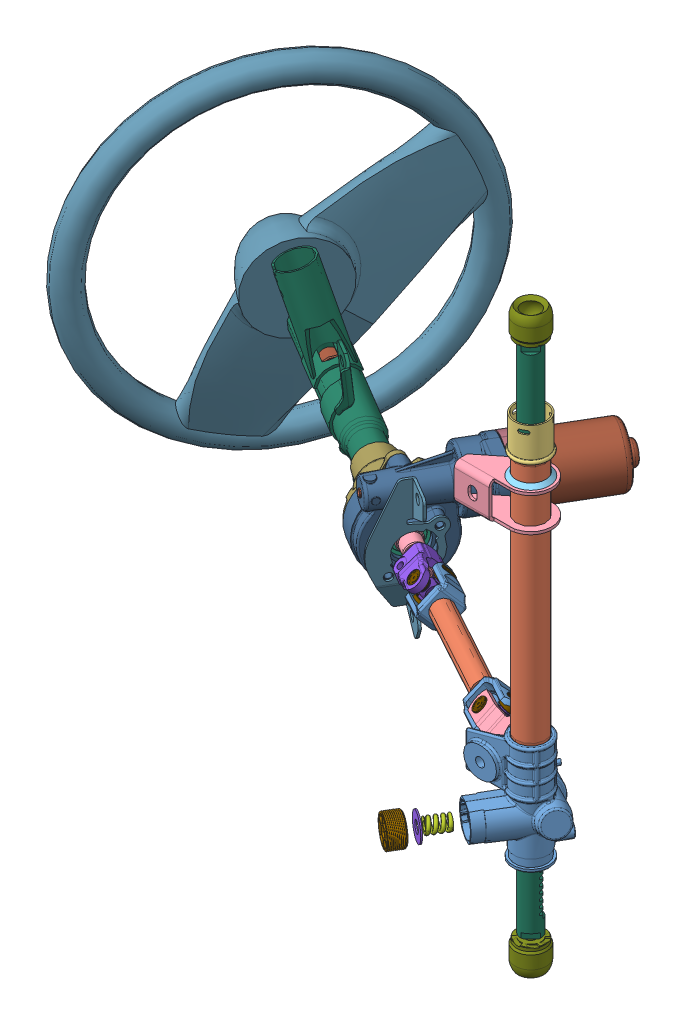
SolidWorks assembly DAE_étude_dynamique, configuration Défaut. Lengths in mm.
Overall size (913.4 791.49 794.04).
64 component instances, 41 part files, 28 mates.
Components (placement in the parent):
- ensemble_carter-1: ensemble_carter [Défaut] at (126.6085 40.308 0) size (712.31 507.21 668.6)
  - ensemble_carter_cremaillere-1: ensemble_carter_cremaillere [Défaut] x (0 1 0) z (0 0 1) size (421.75 126.58 169.81)
    - boitier_pignon-1: boitier_pignon [Défaut] at (-210 0 0) x (1 0 0) z (0 0.523604 0.851962) size (118 84.29 86.02)
    - tube_crémaillère-1: tube_crémaillère [Défaut] at (-128 0 0) x (1 0 0) z (0 0.056204 0.998419) size (305.5 35 35)
    - embout_cremaillere-1: embout_cremaillere [Défaut] at (169.0543 0 0) x (1 0 0) z (0 0.056204 0.998419) size (37.25 39.5 39.5)
    - patte_cremaillere-1: patte_cremaillere [Défaut] at (132 -23 27) x (1 0 0) z (0 1 0) size (40.02 51.5 78)
    - bead2-2: bead2 [Défaut] at origin size (4.91 42.26 42.11)
    - bead3-1: bead3 [Défaut] at origin size (4.91 42.26 42.11)
    - ressort de poussoir-1: ressort de poussoir [Défaut] at (-165 33.9288 55.206) x (1 0 0) z (0 -0.851962 0.523604) size (16.23 26.9 16.26)
    - cale de réglage-1: cale de réglage [Défaut] at (-209.8645 49.6683 74.1505) x (0.996988 -0.066074 0.040608) z (0 0.523604 0.851962) size (28 28 1.4)
    - bouchon de poussoir-1: bouchon de poussoir [Défaut] at (-165 61.4178 99.9336) x (0.75369 0.559935 -0.344128) z (-0.65723 0.642115 -0.394635) size (32.72 18.98 32.65)
  - ensemble_carter_assistance-1: ensemble_carter_assistance [Défaut] at (-346.9207 -175.5297 -314.3536) x (0.861006 0 0.508595) z (-0.508595 0 0.861006) size (350.5 192.4 245.84)
    - carter_réducteur-1: carter_réducteur [Défaut] at origin size (86 132.9 120)
    - boitier_moteur-1: boitier_moteur [Défaut] at (0.008 -0.4901 -13.5) x (0.999849 0.017398 0) z (0 0 1) size (82.29 66 97)
    - carter_capteur-1: carter_capteur [Défaut] at (-24 -42 76) x (1 0 0) z (0 0.868796 -0.49517) size (86 83.51 98.87)
    - flasque_moteur-1: flasque_moteur [Défaut] at (-0.0002 0.0008 -11) x (1 -0.000004 0) z (0 0 1) size (86 66.52 24)
    - tole_pliée-1: tole_pliée [Défaut] at (27.5612 -42 76) x (0 -1 0) z (0 0 1) size (146.94 53.66 68.51)
    - boitier_tole-1: boitier_tole [Défaut] at (-178.9434 -42 76) x (0 0.995099 0.098888) z (-1 0 0) size (176.09 56.57 208)
- ensemble_moteur-1: ensemble_moteur [Défaut] at (-68.4045 -315.0875 -320.7909) x (-0.508595 0 0.861006) z (-0.436791 -0.861768 -0.258012) size (212.24 71.98 71.98)
  - ensemble_embrayage-1: ensemble_embrayage [Défaut] at (103.9489 166.5772 -172.8082) x (-1 0 0) z (0 0.92233 -0.386403) size (22.5 68.3 68.3)
    - moyeu_embrayage-1: moyeu_embrayage [Défaut] at (-3.3483 89.4439 0) size (22.5 30 30)
    - diaphragme_embrayage-1: diaphragme_embrayage [Défaut] at (-3.3483 89.4439 0) x (0 0.866025 0.5) z (-1 0 0) size (50 50 0.5)
    - disque_embrayage-1: disque_embrayage [Défaut] at (-3.3483 89.4439 0) x (0 0 -1) z (1 0 0) size (50 50 2)
  - rotor_moteur-1: rotor_moteur [Défaut] at (-16.0331 201.1386 -90.3114) x (-1 0 0) z (0 0.924225 -0.381849) size (121 46.69 46.69)
  - vis-1: vis [Défaut] at (133.2034 201.1386 -90.3114) x (1 0 0) z (0 0.027722 0.999616) size (88.01 16 16)
  - plateau_embrayage-1: plateau_embrayage [Défaut] at (104.802 201.1386 -90.3114) x (1 0 0) z (0 -0.628921 0.777469) size (17 50 50)
- ensemble_recepteur-1: ensemble_recepteur [Défaut] at (-235.2204 -300.8539 -395.7187) x (-0.861006 0 -0.508595) z (0.338725 0.745951 -0.573431) size (124 97.96 97.96)
  - ensemble_roue-1: ensemble_roue [Défaut] at (-32.6877 82.9298 0) size (91 97.96 97.96)
    - arbre_roue-1: arbre_roue [Défaut] at (-15.5303 102.7038 0) size (88 32 32)
    - creneaux_roue-1: creneaux_roue [Défaut] at (-0.5303 102.7038 0) size (10 31 31)
    - moyeu_roue-1: moyeu_roue [Défaut] at (-27.5303 102.7038 0) x (1 0 0) z (0 -0.027331 0.999626) size (12 62 62)
    - roue-1: roue [Défaut] at (-26.5303 102.7038 0) x (-1 0 0) z (0 0.924225 -0.381849) size (10 75 75)
  - fourche_cardan-1: fourche_cardan [Défaut] at (-93.2179 185.75 -1.9966) x (0 0.998307 0.058156) z (0 -0.058156 0.998307) size (42.34 54.79 32.31)
- ensemble_volant-1: ensemble_volant [Défaut] at (-124.7717 -283.3287 -317.9381) x (-0.861006 0 -0.508595) z (0.338725 0.745951 -0.573431) size (466.36 370 370)
  - barre_de_torsion-1: barre_de_torsion [Défaut] at (165.9378 165.9087 -5.8829) x (1 0 0) z (0 -1 0) size (145 8 8)
  - creneaux_colonne-1: creneaux_colonne [Défaut] at (117.8546 165.9087 -5.8829) x (-1 0 0) z (0 0.979628 -0.200818) size (30 31 31)
  - arbre_trans_ext-1: arbre_trans_ext [Défaut] at (443.3272 165.9087 -5.8829) x (-1 0 0) z (0 0.159988 0.987119) size (204 30 30)
  - arbre_trans_int-1: arbre_trans_int [Défaut] at (179.1633 165.9087 -5.8829) x (1 0 0) z (0 0.159988 0.987119) size (115 17 17)
  - moyeu_de_capteur-1: moyeu_de_capteur [Défaut] at (101.983 165.9087 -5.8829) x (-1 0 0) z (0 0.299586 0.954069) size (88 28 28)
  - volant-1: volant [Défaut] at (470.1285 165.9087 -5.8829) size (73.29 370 370)
- ensemble_cremaillere-1: ensemble_cremaillere [Défaut] at (136.5235 -91.4682 -16.1328) x (0 1 0) z (-0.851962 0 -0.523604) size (625.5 47.69 47.69)
  - Crémaillère-1: Crémaillère [Défaut] at (131.7762 -18.936 0) size (560 22 22)
  - cremaillere_embout-1: cremaillere_embout [Défaut] at (-171.2238 -18.936 0) x (1 0 0) z (0 -0.229093 0.973405) size (45.75 34 34)
  - cremaillere_embout-2: cremaillere_embout [Défaut] at (434.7762 -18.936 0) x (-1 0 0) z (0 -0.791815 -0.610761) size (45.75 34 34)
- ensemble_croisillon-1: ensemble_croisillon [Défaut] at (-153.716 -272.7828 -295.5948) x (-0.359046 0.708255 0.607833) z (0.297668 0.704146 -0.644649) size (40.4 20.18 40.4)
  - croisillon-1: croisillon [Défaut] at (133.8433 15.1586 0) size (36 20 36)
  - roult_aiguilles-1: roult_aiguilles [Défaut] at (113.8433 15.1586 0) x (1 0 0) z (0 -0.005579 0.999984) size (10 15 15)
  - roult_aiguilles-2: roult_aiguilles [Défaut] at (153.8433 15.1586 0) x (-1 0 0) z (0 -0.983447 0.181195) size (10 15 15)
  - roult_aiguilles-3: roult_aiguilles [Défaut] at (133.8433 15.1586 -20) x (0 0 1) z (-0.454157 0.890922 0) size (10 15 15)
  - roult_aiguilles-4: roult_aiguilles [Défaut] at (133.8433 15.1586 20) x (0 0 -1) z (0.994379 0.105875 0) size (10 15 15)
- ensemble_transmission-2: ensemble_transmission [Défaut] at (-25.0759 -155.9976 -108.6312) x (-0.297668 -0.704146 0.644649) z (-0.432992 0.70139 0.566189) size (42 202 30.26)
  - fourche_cardan_3-1: fourche_cardan_3 [Défaut] at origin size (42 79 30.26)
  - arbre_transmission-1: arbre_transmission [Défaut] at origin size (22 150 22)
- ensemble_pignon-1: ensemble_pignon [Défaut] at (190.8525 -108.1522 18.2324) x (0.839019 0.173648 0.515649) z (-0.475407 0.69491 0.539525) size (206.84 48.43 47.04)
  - pignon-1: pignon [Défaut] at (-214.1756 -7.2348 0) size (171 18.5 18.5)
  - fourche_cardan_4-1: fourche_cardan_4 [Défaut] at (-173.9126 -25.7617 0.3119) x (-0.000233 -0.173648 -0.984808) z (-0.999999 0.001339 0) size (40.37 41.95 76.1)
- ensemble_croisillon-2: ensemble_croisillon [Défaut] at (-59.9907 -58.6761 -18.4496) x (0.475407 -0.69491 -0.539525) z (0.297668 0.704146 -0.644649) size (40.4 20.18 40.4)
  - croisillon-1: croisillon [Défaut] at (133.8433 15.1586 0) size (36 20 36)
  - roult_aiguilles-1: roult_aiguilles [Défaut] at (113.8433 15.1586 0) x (1 0 0) z (0 -0.005579 0.999984) size (10 15 15)
  - roult_aiguilles-2: roult_aiguilles [Défaut] at (153.8433 15.1586 0) x (-1 0 0) z (0 -0.983447 0.181195) size (10 15 15)
  - roult_aiguilles-3: roult_aiguilles [Défaut] at (133.8433 15.1586 -20) x (0 0 1) z (-0.454157 0.890922 0) size (10 15 15)
  - roult_aiguilles-4: roult_aiguilles [Défaut] at (133.8433 15.1586 20) x (0 0 -1) z (0.994379 0.105875 0) size (10 15 15)
- fourche_cardan_3-2: fourche_cardan_3 [Défaut] at (-172.1971 -175.1205 -197.4526) x (0.297668 0.704146 -0.644649) z (-0.432992 0.70139 0.566189) size (42 79 30.26)
- poussoir-1: poussoir [Défaut] at (153.5095 -124.692 -43.771) x (0 -1 0) z (-0.851962 0 -0.523604) size (28 28 28)
Mates (geometry in assembly coordinates):
- Coaxialité crémaillère corps: concentric anti-aligned: cylinder of ensemble_carter-1/ensemble_carter_cremaillere-1/tube_crémaillère-1 through (126.6085 -87.692 0) axis (0 -1 0) radius 16; cylinder of ensemble_cremaillere-1/Crémaillère-1 through (126.6085 341.308 0) axis (0 1 0) radius 11
- Parallèle orientation angulaire crémaillère corps: parallel anti-aligned: plane of ensemble_carter-1/ensemble_carter_cremaillere-1/boitier_pignon-1 through (131.8445 -169.692 -8.5196) normal (-0.523604 0 0.851962); plane of ensemble_cremaillere-1/Crémaillère-1 through (141.4469 -222.2361 -0.2706) normal (0.523604 0 -0.851962)
- Coaxialité croisillon supérieur / récepteur: unknown anti-aligned: cylinder of ensemble_recepteur-1/fourche_cardan-1 through (-195.964 -162.2277 -194.3443) axis (0.359046 -0.708255 -0.607833) radius 7; cylinder of ensemble_croisillon-1/roult_aiguilles-2 through (-195.5438 -163.0566 -195.0557) axis (-0.359046 0.708255 0.607833) radius 7.5
- Position axiale croisillon supérieur / récepteur: coincident aligned: plane of ensemble_recepteur-1/fourche_cardan-1; plane of ensemble_croisillon-1/croisillon-1
- Coaxialité pignon / corps: unknown aligned: cylinder of ensemble_carter-1/ensemble_carter_cremaillere-1/boitier_pignon-1 through (88.3032 -134.0287 -38.8008) axis (-0.839019 -0.173648 -0.515649) radius 16; cylinder of ? through (9.2406 -150.3919 -87.3916) axis (-0.839019 -0.173648 -0.515649) radius 9
- distance arrêt en translation pignon / corps: distance = 8 mm anti-aligned: plane of ensemble_carter-1/ensemble_carter_cremaillere-1/boitier_pignon-1 through (101.6747 -133.3744 -53.4712) normal (-0.839019 -0.173648 -0.515649); plane of ensemble_pignon-1/pignon-1 through (87.2002 -128.3088 -47.1399) normal (0.839019 0.173648 0.515649)
- Coaxialité croisillon inférieur / pignon: unknown aligned: cylinder of ? through (-17.6533 -141.1162 -88.949) axis (0.475407 -0.69491 -0.539525) radius 7.5; cylinder of ? through (0.5981 -167.7946 -109.662) axis (0.475407 -0.69491 -0.539525) radius 7.5
- Position axiale croisillon inférieur / pignon: unknown anti-aligned: plane of ? through (190.8525 -108.1522 18.2324) normal (-0.475407 0.69491 0.539525); unknown of ?
- Coaxialité croisillon supérieur / inter: unknown anti-aligned: cylinder of ensemble_croisillon-1/roult_aiguilles-3 through (-194.3163 -191.3046 -194.3193) axis (-0.297668 -0.704146 0.644649) radius 7.5; cylinder of fourche_cardan_3-2 through (-195.8046 -194.8253 -191.0961) axis (0.297668 0.704146 -0.644649) radius 7.5
- Position axiale croisillon supérieur / inter: unknown aligned: plane of ensemble_croisillon-1/croisillon-1 through (-188.3629 -177.2217 -207.2123) normal (0.297668 0.704146 -0.644649); unknown of fourche_cardan_3-2
- Coaxialité croisillon inférieur / inter: unknown aligned: cylinder of ? through (-1.4684 -136.2927 -114.9877) axis (-0.297668 -0.704146 0.644649) radius 7.5; cylinder of ? through (-14.8634 -167.9793 -85.9785) axis (-0.297668 -0.704146 0.644649) radius 7.5
- Position axiale croisillon inférieur / inter: unknown anti-aligned: unknown of ?; plane of ? through (-8.9101 -153.8964 -98.8715) normal (0.297668 0.704146 -0.644649)
- Coaxialité arbre de transmission / cardan inférieur: unknown anti-aligned: cylinder of ? through (-25.0759 -155.9976 -108.6312) axis (0.85083 0.110591 0.513671) radius 9; cylinder of fourche_cardan_3-2 through (-172.1971 -175.1205 -197.4526) axis (-0.85083 -0.110591 -0.513671) radius 9
- Position angulaire arbre de transmission / cardan inférieur: unknown aligned: plane of ? through (-25.0759 -155.9976 -108.6312) normal (-0.432992 0.70139 0.566189); plane of fourche_cardan_3-2 through (-172.1971 -175.1205 -197.4526) normal (-0.432992 0.70139 0.566189)
- Coaxialité récpteur / carter: unknown anti-aligned: cylinder of ensemble_carter-1/ensemble_carter_assistance-1/carter_réducteur-1 through (-218.9286 -177.2217 -225.2674) axis (0.861006 0 0.508595) radius 21; cylinder of ensemble_recepteur-1/ensemble_roue-1/arbre_roue-1 through (-296.8496 -177.2217 -271.2953) axis (-0.861006 0 -0.508595) radius 10
- Position axiale récepteur / carter: unknown aligned: plane of ensemble_carter-1/ensemble_carter_assistance-1/carter_réducteur-1 through (-246.9113 -156.2217 -241.7968) normal (0.861006 0 0.508595); plane of ensemble_recepteur-1/ensemble_roue-1/arbre_roue-1 through (-251.0846 -169.8957 -234.7318) normal (0.861006 0 0.508595)
- Coaxialité volant / carter: unknown anti-aligned: cylinder of ensemble_carter-1/ensemble_carter_assistance-1/boitier_tole-1 through (-413.0367 -177.2217 -339.9268) axis (0.861006 0 0.508595) radius 18.5; cylinder of ensemble_volant-1/arbre_trans_ext-1 through (-578.3033 -177.2217 -437.5496) axis (-0.861006 0 -0.508595) radius 10
- coaxialité goupille barre de torsion recepteur: unknown aligned: cylinder of ensemble_recepteur-1/ensemble_roue-1/arbre_roue-1 through (-217.8907 -189.1569 -212.2781) axis (0.338725 0.745951 -0.573431) radius 2; cylinder of ensemble_volant-1/barre_de_torsion-1 through (-213.826 -180.2055 -219.1593) axis (0.338725 0.745951 -0.573431) radius 2
- Coaxial3: unknown anti-aligned: cylinder of ensemble_carter-1/ensemble_carter_assistance-1/flasque_moteur-1 through (-236.5695 -135.2218 -286.8317) axis (-0.508595 0 0.861006) radius 11.0009; cylinder of ensemble_moteur-1/vis-1 through (-229.1625 -135.2218 -299.371) axis (0.508595 0 -0.861006) radius 4.5
- A distance2: unknown = 7 mm anti-aligned: plane of ensemble_carter-1/ensemble_carter_assistance-1/flasque_moteur-1 through (-219.2951 -126.2209 -316.0756) normal (-0.508595 0 0.861006); plane of ensemble_moteur-1/plateau_embrayage-1 through (-225.8358 -135.7383 -311.8092) normal (0.508595 0 -0.861006)
- Coïncidente8: unknown: point of ensemble_carter-1; unknown of ensemble_cremaillere-1/Crémaillère-1
- Coaxial6: unknown anti-aligned: cylinder of ensemble_carter-1/ensemble_carter_cremaillere-1/boitier_pignon-1 through (104.0351 -124.692 36.7294) axis (-0.523604 0 0.851962) radius 15; cylinder of poussoir-1 through (145.7563 -124.692 -31.1555) axis (0.523604 0 -0.851962) radius 14
- Parallèle1: unknown anti-aligned: axis of ensemble_carter-1/ensemble_carter_cremaillere-1/boitier_pignon-1 through (126.6085 -185.692 0) axis (0 1 0); line of poussoir-1 through (118.1849 -111.0172 7.9766) axis (0 -1 0)
- Coïncidente9: unknown anti-aligned: plane of ensemble_carter-1/ensemble_carter_cremaillere-1/ressort de poussoir-1 through (92.6797 -124.692 55.206) normal (0.851962 0 0.523604); plane of poussoir-1 through (153.5095 -124.692 -43.771) normal (-0.851962 0 -0.523604)
- Coïncidente10: unknown anti-aligned: unknown of ensemble_carter-1/ensemble_carter_cremaillere-1/ressort de poussoir-1; unknown of poussoir-1
- Coaxial7: unknown aligned: cylinder of ensemble_carter-1/ensemble_carter_cremaillere-1/cale de réglage-1 through (79.1805 -124.692 77.1707) axis (0.523604 0 -0.851962) radius 14; cylinder of poussoir-1 through (145.7563 -124.692 -31.1555) axis (0.523604 0 -0.851962) radius 14
- Tangent1: tangent anti-aligned: cylinder of ensemble_cremaillere-1/Crémaillère-1 through (126.6085 341.308 0) axis (0 1 0) radius 11; sphere of poussoir-1
- Tangent2: tangent anti-aligned: cylinder of ensemble_cremaillere-1/Crémaillère-1 through (126.6085 341.308 0) axis (0 1 0) radius 11; sphere of poussoir-1
